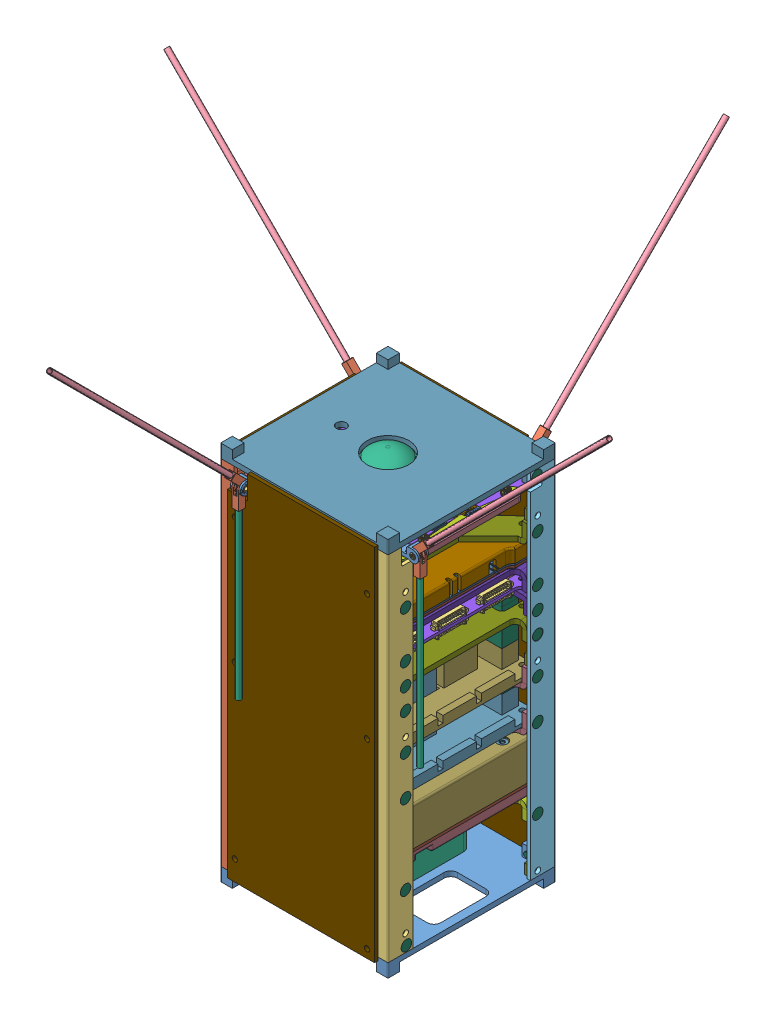
SolidWorks assembly Cubesat, configuration Default. Lengths in mm. (continued)
Mates (geometry in assembly coordinates):
- Coincident3: coincident: point of Cover Plate Bottom-1; point of assembly
- Coincident4: coincident: plane of Cover Plate Bottom-1 through (0 0 0) normal (0 -1 0); plane of assembly through (0 0 0) normal (0 1 0)
- Coincident5: coincident: plane of Cover Plate Bottom-1 through (0 0 0) normal (0 0 1); plane of assembly through (0 0 0) normal (0 0 1)
- Coincident7: coincident: plane of Cover Plate Bottom-1 through (0 0 0) normal (0 1 0); plane of Rail - Top Left-1 through (-50 0 -35) normal (0 -1 0)
- Coincident8: coincident: plane of Rail - Top Left-1 through (-50 211 -35) normal (0 0 1); plane of Cover Plate Bottom-1 through (-48 7 -35) normal (0 0 1)
- Coincident10: coincident: plane of Cover Plate Bottom-1 through (0 0 0) normal (0 1 0); plane of Rail - Top Right-1 through (35 0 -35) normal (0 -1 0)
- Coincident12: coincident: plane of Cover Plate Bottom-1 through (43 7 -48) normal (0 0 -1); plane of Rail - Top Right-1 through (35 211 -48) normal (0 0 1)
- Coincident13: coincident: plane of Cover Plate Bottom-1 through (0 0 0) normal (0 1 0); plane of Rail - Bottom Left-1 through (-50 0 50) normal (0 -1 0)
- Coincident14: coincident: plane of Cover Plate Bottom-1 through (-35 7 48) normal (0 0 1); plane of Rail - Bottom Left-1 through (-50 211 48) normal (0 0 -1)
- Coincident16: coincident: plane of Cover Plate Bottom-1 through (0 0 0) normal (0 1 0); plane of Rail - Bottom Right-1 through (50 0 50) normal (0 -1 0)
- Coincident18: coincident: plane of Rail - Bottom Right-1 through (50 211 35) normal (0 0 -1); plane of Cover Plate Bottom-1 through (48 7 35) normal (0 0 -1)
- Concentric1: concentric: circle of Camera-1; cylinder of Camera Plate - 4 tabs - bottom-1 through (-22.0002 39.32 -22.0002) axis (0 1 0) radius 1.7
- Concentric2: concentric: cylinder of Camera-1 through (22.0002 28.82 22.0002) axis (0 1 0) radius 1.5; cylinder of Camera Plate - 4 tabs - bottom-1 through (22.0002 39.32 22.0002) axis (0 1 0) radius 1.7
- Coincident19: coincident: plane of Camera-1 through (0 36.32 0) normal (0 1 0); plane of Camera Plate - 4 tabs - bottom-1 through (0 36.32 0) normal (0 -1 0)
- Concentric4: concentric: cylinder of Cover Plate Bottom-1 through (0 -3 0) axis (0 1 0) radius 12.5; cylinder of Camera-1 through (0 9.82 0) axis (0 1 0) radius 11.5307
- Distance2: distance = 2 mm: plane of Camera-1 through (0 -6 0) normal (0 -1 0); plane of Cover Plate Bottom-1 through (0 -8 0) normal (0 -1 0)
- Coincident30: coincident: plane of Camera Plate - 4 tabs - bottom-1 through (0 39.32 0) normal (0 1 0); plane of EPS1+-1/EPS1+.STEP-1/bottom-cover_Rev1.2.STEP-1 through (0 39.32 0) normal (0 -1 0)
- Concentric6: concentric: circle of Camera Plate - 4 tabs - bottom-1; circle of EPS1+-1/EPS1+.STEP-1/top-cover.STEP-1
- Concentric7: concentric: circle of Camera Plate - 4 tabs - bottom-1; circle of EPS1+-1/EPS1+.STEP-1/top-cover.STEP-1
- Coincident33: coincident: plane of Rail - Top Left-1 through (-48 211 -35) normal (1 0 0); plane of Camera Plate - 4 tabs - bottom-1 through (-48 39.32 0) normal (-1 0 0)
- Coincident37: coincident: plane of Camera-2 through (0 174.68 0) normal (0 -1 0); plane of Camera Plate - 4 tabs - top-1 through (0 174.68 0) normal (0 1 0)
- Coincident40: coincident: plane of Rail - Top Left-1 through (-48 211 -35) normal (1 0 0); plane of Camera Plate - 4 tabs - top-1 through (-48 174.68 0) normal (-1 0 0)
- Concentric10: concentric: cylinder of Camera-2 through (-22.0002 182.18 -22.0002) axis (0 -1 0) radius 1.5; cylinder of Camera Plate - 4 tabs - top-1 through (-22.0002 171.68 -22.0002) axis (0 1 0) radius 1.55
- Concentric13: concentric: circle of Camera Plate - 4 tabs - top-1; circle of OBC_EnduroSat-1/OBC_EnduroSat.STEP-1/Board021117.STEP-1
- Concentric14: concentric: cylinder of Camera Plate - 4 tabs - top-1 through (37.5 171.68 -42.85) axis (0 1 0) radius 1.55; circle of OBC_EnduroSat-1/OBC_EnduroSat.STEP-1/Board021117.STEP-1
- Concentric15: concentric: cylinder of Camera Plate - 4 tabs - top-1 through (-36.2 171.68 -42.85) axis (0 1 0) radius 1.55; cylinder of UHF_comm_type_II-1/UHF_comm_type_II.STEP-1/UHF_BOX.STEP-1 through (-36.2 168.68 -42.85) axis (0 -1 0) radius 1.6
- Concentric16: concentric: cylinder of Camera Plate - 4 tabs - top-1 through (37.5 171.68 -42.85) axis (0 1 0) radius 1.55; cylinder of UHF_comm_type_II-1/UHF_comm_type_II.STEP-1/UHF_BOX.STEP-1 through (37.5 168.68 -42.85) axis (0 -1 0) radius 1.6
- Distance4: distance = 24 mm: plane of OBC_EnduroSat-1/OBC_EnduroSat.STEP-1/Board021117.STEP-1 through (42.1 144.68 47.95) normal (0 -1 0); plane of UHF_comm_type_II-1/UHF_comm_type_II.STEP-1/UHF_BOX.STEP-1 through (40.1038 168.68 -45.05) normal (0 1 0)
- Distance5: distance = 6 mm: plane of UHF_comm_type_II-1/UHF_comm_type_II.STEP-1/UHF_BOX.STEP-1 through (40.1038 168.68 -45.05) normal (0 1 0); plane of Camera-2 through (0 174.68 0) normal (0 -1 0)
- Concentric17: concentric: cylinder of Custom Board 2-1 through (-36.2 77.989 -42.85) axis (0 -1 0) radius 1.6; cylinder of Custom Board 1 Plate-2 through (-36.2 72.989 -42.85) axis (0 1 0) radius 1.55
- Concentric18: concentric: cylinder of Custom Board 2-1 through (40 77.989 42.85) axis (0 -1 0) radius 1.6; circle of Custom Board 1 Plate-2
- Coincident49: coincident: plane of Custom Board 2-1 through (0 75.989 0) normal (0 -1 0); plane of Custom Board 1 Plate-2 through (0 75.989 0) normal (0 1 0)
- Concentric19: concentric: circle of Custom Board 1-1; cylinder of Custom Board 1 Plate-1 through (-36.2 96.589 -42.85) axis (0 1 0) radius 1.55
- Concentric20: concentric: cylinder of Custom Board 1-1 through (40 101.589 42.85) axis (0 -1 0) radius 1.6; cylinder of Custom Board 1 Plate-1 through (40 96.589 42.85) axis (0 1 0) radius 1.55
- Coincident51: coincident: plane of Custom Board 1-1 through (0 99.589 0) normal (0 -1 0); plane of Custom Board 1 Plate-1 through (0 99.589 0) normal (0 1 0)
- Coincident54: coincident: plane of EPS1+-1/EPS1+.STEP-1/ESQ_126_69_G_D.STEP-1/_ESQ_126_69_G_D_socket_2.STEP-1 through (-32.6249 65.189 -36.5581) normal (0 1 0); plane of PC104 Connector-1 through (-32.6269 65.189 -34.0211) normal (0 -1 0)
- Coincident55: coincident: plane of EPS1+-1/EPS1+.STEP-1/ESQ_126_69_G_D.STEP-2/_ESQ_126_69_G_D_socket_2.STEP-1 through (33.9231 65.189 -44.0511) normal (0 0 -1); plane of PC104 Connector-1 through (-32.6269 75.989 -44.0511) normal (0 0 -1)
- Coincident56: coincident: plane of EPS1+-1/EPS1+.STEP-1/ESQ_126_69_G_D.STEP-2/_ESQ_126_69_G_D_socket_2.STEP-1 through (33.9231 65.189 -39.0981) normal (1 0 0); plane of PC104 Connector-1 through (33.9231 75.989 -34.0211) normal (1 0 0)
- Concentric21: concentric: circle of EPS1+-1/EPS1+.STEP-1/top-cover.STEP-1; cylinder of Custom Board 2-1 through (37.5 77.989 -42.85) axis (0 -1 0) radius 1.6
- Coincident58: coincident: plane of Rail - Bottom Left-1 through (-48 211 50) normal (1 0 0); plane of Custom Board 1 Plate-2 through (-48 75.989 0) normal (-1 0 0)
- Coincident63: coincident: plane of Custom Board 2-1 through (0 75.989 0) normal (0 -1 0); plane of PC104 Connector-1 through (-32.6269 75.989 -34.0211) normal (0 1 0)
- Concentric22: concentric: circle of Custom Board 1-1; circle of Custom Board 2-1
- Coincident61: coincident: plane of Rail - Bottom Left-1 through (-48 211 50) normal (1 0 0); plane of Custom Board 1 Plate-1 through (-48 99.589 0) normal (-1 0 0)
- Coincident64: coincident: plane of Custom Board 2-1 through (0 88.789 0) normal (0 1 0); plane of PC104 Connector-2 through (-32.627 88.789 -34.051) normal (0 -1 0)
- Coincident65: coincident: plane of Custom Board 2-1 through (33.923 88.789 -44.081) normal (1 0 0); plane of PC104 Connector-2 through (33.923 99.589 -34.051) normal (1 0 0)
- Coincident66: coincident: plane of Custom Board 2-1 through (-32.625 88.789 -44.081) normal (0 0 -1); plane of PC104 Connector-2 through (-32.627 99.589 -44.081) normal (0 0 -1)
- Coincident67: coincident: plane of Custom Board 1-1 through (0 99.589 0) normal (0 -1 0); plane of PC104 Connector-2 through (-32.627 99.589 -34.051) normal (0 1 0)
- Coincident70: coincident: plane of Custom Board 1-1 through (0 112.389 0) normal (0 1 0); plane of PC104 Connector-4 through (-32.627 112.389 -34.112) normal (0 -1 0)
- Coincident71: coincident: plane of Custom Board 1-1 through (33.923 112.389 -44.091) normal (1 0 0); plane of PC104 Connector-4 through (33.923 123.189 -34.112) normal (1 0 0)
- Coincident73: coincident: plane of Custom Board 1-1 through (-32.625 112.389 -34.112) normal (0 0 1); plane of PC104 Connector-4 through (-32.627 123.189 -34.112) normal (0 0 1)
- Coincident74: coincident: plane of PC104 Connector-4 through (-32.627 123.189 -34.112) normal (0 1 0); plane of PC104 Connector-5 through (-32.627 123.189 -34.112) normal (0 -1 0)
- Coincident75: coincident: plane of PC104 Connector-4 through (33.923 123.189 -34.112) normal (1 0 0); plane of PC104 Connector-5 through (33.923 133.989 -34.112) normal (1 0 0)
- Coincident76: coincident: plane of Custom Board 1-1 through (-32.625 112.389 -34.112) normal (0 0 1); plane of PC104 Connector-5 through (-32.627 133.989 -34.112) normal (0 0 1)
- Coincident77: coincident: plane of PC104 Connector-3 through (-32.627 133.989 -34.112) normal (0 -1 0); plane of PC104 Connector-5 through (-32.627 133.989 -34.112) normal (0 1 0)
- Coincident78: coincident: plane of PC104 Connector-3 through (33.923 144.789 -34.112) normal (1 0 0); plane of PC104 Connector-5 through (33.923 133.989 -34.112) normal (1 0 0)
- Coincident79: coincident: plane of PC104 Connector-3 through (-32.627 144.789 -44.142) normal (0 0 -1); plane of PC104 Connector-5 through (-32.627 133.989 -44.142) normal (0 0 -1)
- Coincident82: coincident: plane of Rail - Top Left-1 through (-48 211 -35) normal (1 0 0); plane of Engraving plate-1 through (-48 131.989 0) normal (-1 0 0)
- Concentric25: concentric: cylinder of Custom Board 1-1 through (40 101.589 42.85) axis (0 -1 0) radius 1.6; circle of Engraving plate-1
- Distance7: distance = 1 mm: plane of Custom Board 2-1 through (0 127.989 0) normal (0 1 0); plane of Engraving plate-1 through (0 128.989 0) normal (0 -1 0)
- Coincident84: coincident: plane of Rail - Bottom Left-1 through (-48 211 50) normal (1 0 0); plane of OBC Board Plate-1 through (-48 144.68 0) normal (-1 0 0)
- Coincident85: coincident: plane of OBC_EnduroSat-1/OBC_EnduroSat.STEP-1/Board021117.STEP-1 through (42.1 144.68 47.95) normal (0 -1 0); plane of OBC Board Plate-1 through (0 144.68 0) normal (0 1 0)
- Concentric27: concentric: circle of Engraving plate-1; circle of Engraving-1
- Concentric28: concentric: circle of Engraving plate-1; circle of Engraving-1
- Coincident86: coincident: plane of Engraving plate-1 through (0 131.989 0) normal (0 1 0); plane of Engraving-1 through (0 131.989 0) normal (0 -1 0)
- Concentric30: concentric: circle of gs-3dcad-nanocom-ant430-2u3u-deployed-4-1/panel-top_ant430-2U-4-1; circle of Antenna Plate-1
- Concentric31: concentric: cylinder of gs-3dcad-nanocom-ant430-2u3u-deployed-4-1/2.5x4.5x3.0mm-spacer_ant430-2U-4-4 through (-45.8 206 24.7) axis (0 -1 0) radius 1.25; cylinder of Antenna Plate-1 through (-45.8 192 24.7) axis (0 1 0) radius 1.35
- Coincident87: coincident: plane of gs-3dcad-nanocom-ant430-2u3u-deployed-4-1/panel-top_ant430-2U-4-1 through (47.4 202 -32.35) normal (0 -1 0); plane of Antenna Plate-1 through (0 202 0) normal (0 1 0)
- Coincident88: coincident: plane of Rail - Bottom Left-1 through (-50 211 48) normal (0 0 -1); plane of Antenna Plate-1 through (0 202 48) normal (0 0 1)
- Coincident110: coincident: plane of Rail - Bottom Right-1 through (50 211 50) normal (0 1 0); plane of Cover Plate Top-2 through (0 211 0) normal (0 -1 0)
- Coincident111: coincident: plane of Rail - Bottom Right-1 through (50 211 48) normal (0 0 -1); plane of Cover Plate Top-2 through (35 204 48) normal (0 0 1)
- Coincident112: coincident: plane of Rail - Top Right-1 through (48 211 -35) normal (-1 0 0); plane of Cover Plate Top-2 through (48 204 -35) normal (1 0 0)
- Coincident113: coincident: plane of Rail - Bottom Right-1 through (35 211 50) normal (-1 0 0); plane of Antenna Plate-1 through (35 192 48) normal (-1 0 0)
- Concentric32: concentric: cone of Rail - Bottom Left-1 through (-50 178.5483 39.5) axis (1 0 0); cone of M3 Flathead-3 through (-50 178.5483 39.5) axis (1 0 0)
- Coincident116: coincident: circle of Rail - Bottom Left-1; cone of M3 Flathead-1 through (-50 150.8117 39.5) axis (1 0 0)
- Coincident117: coincident: circle of Rail - Bottom Left-1; circle of M3 Flathead-8
- Coincident118: coincident: circle of Rail - Bottom Left-1; circle of M3 Flathead-5
- Coincident119: coincident: circle of Rail - Bottom Left-1; circle of M3 Flathead-7
- Coincident120: coincident: circle of Rail - Bottom Left-1; circle of M3 Flathead-2
- Coincident121: coincident: circle of Rail - Top Left-1; cone of M3 Flathead-6 through (-50 178.5483 -39.5) axis (1 0 0)
- Coincident122: coincident: circle of Rail - Top Left-1; cone of M3 Flathead-4 through (-49.8242 150.8117 -39.5) axis (1 0 0)
- Concentric33: concentric: cone of Rail - Top Left-1 through (-50 137.8117 -39.5) axis (1 0 0); cone of M3 Flathead-12 through (-50 137.8117 -39.5) axis (1 0 0)
- Coincident124: coincident: circle of Rail - Top Left-1; circle of M3 Flathead-11
- Coincident125: coincident: circle of Rail - Top Left-1; circle of M3 Flathead-9
- Coincident126: coincident: circle of Rail - Top Left-1; circle of M3 Flathead-10
- Coincident127: coincident: circle of Rail - Top Left-1; circle of M3 Flathead-13
- Coincident128: coincident: circle of Rail - Bottom Right-1; circle of M3 Flathead-14
- Coincident129: coincident: circle of Rail - Top Right-1; circle of M3 Flathead-15
- Coincident130: coincident: circle of Rail - Bottom Right-1; circle of M3 Flathead-16
- Coincident131: coincident: circle of Rail - Top Right-1; circle of M3 Flathead-17
- Coincident132: coincident: circle of Rail - Bottom Right-1; circle of M3 Flathead-18
- Coincident133: coincident: circle of Rail - Top Right-1; circle of M3 Flathead-19
- Coincident134: coincident: circle of Rail - Bottom Right-1; circle of M3 Flathead-20
- Coincident135: coincident: circle of Rail - Top Right-1; cone of M3 Flathead-21 through (49.8242 125.1207 -39.5) axis (-1 0 0)
- Coincident136: coincident: cone of Rail - Bottom Right-1 through (50 103.5207 39.5) axis (-1 0 0); circle of M3 Flathead-22
- Concentric34: concentric: cone of Rail - Top Right-1 through (50 103.4607 -39.5) axis (-1 0 0); cone of M3 Flathead-23 through (50 103.4607 -39.5) axis (-1 0 0)
- Coincident137: coincident: circle of Rail - Bottom Right-1; circle of M3 Flathead-24
- Coincident138: coincident: circle of Rail - Top Right-1; circle of M3 Flathead-26
- Concentric36: concentric: cone of Rail - Bottom Right-1 through (50 32.5107 39.5) axis (-1 0 0); cone of M3 Flathead-25 through (50 32.5107 39.5) axis (-1 0 0)
- Concentric38: concentric: cone of Rail - Top Left-1 through (-39 207.5 -50) axis (0 0 1); cone of M3 Flathead-28 through (-39 207.5 -50) axis (0 0 1)
- Concentric39: concentric: cone of Rail - Bottom Left-1 through (-50 207.5 39) axis (1 0 0); cone of M3 Flathead-29 through (-50 207.5 39) axis (1 0 0)
- Concentric40: concentric: cone of Rail - Top Right-1 through (50 207.5 -39) axis (-1 0 0); cone of M3 Flathead-30 through (50 207.5 -39) axis (-1 0 0)
- Concentric41: concentric: cone of Rail - Bottom Right-1 through (39 207.5 50) axis (0 0 -1); cone of M3 Flathead-31 through (39 207.5 50) axis (0 0 -1)
- Coincident139: coincident: plane of Rail - Bottom Right-1 through (50 211 35) normal (0 0 -1); plane of Cover Plate Bottom-1 through (48 7 35) normal (0 0 -1)
- Coincident140: coincident: plane of Cover Plate Bottom-1 through (35 7 -48) normal (-1 0 0); plane of Rail - Top Right-1 through (35 211 -35) normal (-1 0 0)
- Concentric42: concentric: circle of Camera-2; circle of Camera Plate - 4 tabs - top-1
- Concentric43: concentric: cylinder of Camera Plate - 4 tabs - top-1 through (-40 171.68 42.85) axis (0 1 0) radius 1.55; cylinder of Engraving plate-1 through (-40 128.989 42.85) axis (0 1 0) radius 1.6
- Distance8: distance = 2 mm: plane of Camera-2 through (0 217 0) normal (0 1 0); plane of Cover Plate Top-2 through (0 219 0) normal (0 1 0)
- Concentric44: concentric: cylinder of Engraving plate-1 through (-40 128.989 42.85) axis (0 1 0) radius 1.6; cylinder of OBC Board Plate-1 through (-40 141.68 42.85) axis (0 1 0) radius 1.55
- Coincident141: coincident: cone of Rail - Top Right-1 through (50 32.4507 -39.5) axis (-1 0 0); circle of M3 Flathead-27
- Coincident142: coincident: plane of Cover Plate Bottom-1 through (48 7 35) normal (1 0 0); plane of Rail - Bottom Right-1 through (48 211 50) normal (-1 0 0)
- Distance9: distance = 1 mm: plane of Rail - Top Right-1 through (35 201 -35) normal (0 1 0); plane of gs-3dcad-nanocom-ant430-2u3u-deployed-4-1/panel-top_ant430-2U-4-1 through (47.4 202 -32.35) normal (0 -1 0)
- Coincident143: coincident: circle of Rail - Bottom Left-1; circle of M3 Flathead-32
- Coincident144: coincident: circle of Rail - Bottom Right-1; circle of M3 Flathead-33
- Coincident145: coincident: circle of Rail - Top Right-1; circle of M3 Flathead-34
- Coincident146: coincident: circle of Rail - Top Left-1; circle of M3 Flathead-35
- Coincident147: coincident: circle of Rail - Bottom Left-1; circle of M3 Flathead-36
- Coincident156: coincident: plane of Cover Plate Bottom-1 through (0 7 0) normal (0 1 0); plane of M3 Square Nut-29 through (48 7 42.5) normal (0 -1 0)
- Coincident157: coincident: plane of Cover Plate Bottom-1 through (0 0 0) normal (0 1 0); plane of M3 Square Nut-25 through (48 0 -36.5) normal (0 -1 0)
- Coincident158: coincident: plane of Custom Board 1 Plate-1 through (48 108.589 35) normal (0 1 0); plane of M3 Square Nut-30 through (48 108.589 36.5) normal (0 -1 0)
- Coincident160: coincident: plane of Camera Plate - 4 tabs - top-1 through (48 183.68 44) normal (0 1 0); plane of M3 Square Nut-32 through (48 183.68 42.5) normal (0 -1 0)
- Coincident161: coincident: plane of Camera Plate - 4 tabs - top-1 through (48 183.68 -35) normal (0 1 0); plane of M3 Square Nut-28 through (48 183.68 -36.5) normal (0 -1 0)
- Coincident163: coincident: plane of Custom Board 1 Plate-1 through (48 108.589 -44) normal (0 1 0); plane of M3 Square Nut-26 through (48 108.589 -36.5) normal (0 -1 0)
- Coincident164: coincident: plane of M3 Square Nut-21 through (-45 0 36.5) normal (0 -1 0); plane of Cover Plate Bottom-1 through (0 0 0) normal (0 1 0)
- Coincident165: coincident: plane of Cover Plate Bottom-1 through (0 7 0) normal (0 1 0); plane of M3 Square Nut-17 through (-48 7 -36.5) normal (0 -1 0)
- Coincident166: coincident: plane of Custom Board 1 Plate-1 through (-48 108.589 35) normal (0 1 0); plane of M3 Square Nut-22 through (-48 108.589 42.5) normal (0 -1 0)
- Coincident167: coincident: plane of Custom Board 1 Plate-1 through (-48 108.589 -35) normal (0 1 0); plane of M3 Square Nut-18 through (-48 108.589 -36.5) normal (0 -1 0)
- Coincident170: coincident: plane of Camera Plate - 4 tabs - top-1 through (-48 183.68 35) normal (0 1 0); plane of M3 Square Nut-24 through (-45 183.68 36.5) normal (0 -1 0)
- Coincident171: coincident: plane of Camera Plate - 4 tabs - top-1 through (-48 183.68 -44) normal (0 1 0); plane of M3 Square Nut-20 through (-48 183.68 -42.5) normal (0 -1 0)
- Coincident175: coincident: plane of Rail - Top Right-1 through (48 211 -35) normal (-1 0 0); plane of M3 Square Nut-28 through (48 183.68 -36.5) normal (1 0 0)
- Coincident176: coincident: plane of Camera Plate - 4 tabs - top-1 through (48 174.68 0) normal (1 0 0); plane of M3 Square Nut-32 through (48 183.68 42.5) normal (1 0 0)
- Coincident179: coincident: plane of Custom Board 1 Plate-2 through (48 75.989 0) normal (1 0 0); plane of M3 Square Nut-30 through (48 114.589 36.5) normal (1 0 0)
- Coincident180: coincident: plane of Rail - Top Right-1 through (48 211 -35) normal (-1 0 0); plane of M3 Square Nut-26 through (48 114.589 -36.5) normal (1 0 0)
- Coincident181: coincident: plane of Cover Plate Bottom-1 through (48 7 35) normal (1 0 0); plane of M3 Square Nut-29 through (48 13 42.5) normal (1 0 0)
- Coincident182: coincident: plane of Rail - Top Right-1 through (48 211 -35) normal (-1 0 0); plane of M3 Square Nut-25 through (48 0 -36.5) normal (1 0 0)
- Coincident183: coincident: plane of UHF_comm_type_II-1/UHF_comm_type_II.STEP-1/UHF_BOX-bottom-part(nif).STEP-1 through (44.4 157.68 33.95) normal (0 -1 0); plane of Custom Plate - tabs down-1 through (0 157.68 0) normal (0 1 0)
- Concentric47: concentric: cylinder of UHF_comm_type_II-1/UHF_comm_type_II.STEP-1/UHF_BOX-bottom-part(nif).STEP-1 through (-40 159.68 42.85) axis (0 -1 0) radius 1.6; cylinder of Custom Plate - tabs down-1 through (-40 154.68 42.85) axis (0 1 0) radius 1.55
- Concentric48: concentric: cylinder of UHF_comm_type_II-1/UHF_comm_type_II.STEP-1/UHF_BOX-bottom-part(nif).STEP-1 through (-36.2 157.68 -42.85) axis (0 1 0) radius 1.6; circle of Custom Plate - tabs down-1
- Coincident184: coincident: plane of Rail - Top Left-1 through (-48 211 -35) normal (1 0 0); plane of M3 Square Nut-17 through (-48 7 -36.5) normal (-1 0 0)
- Coincident185: coincident: plane of M3 Square Nut-17 through (-48 7 -36.5) normal (-1 0 0); plane of M3 Square Nut-21 through (-48 6 36.5) normal (-1 0 0)
- Coincident186: coincident: plane of Custom Board 1 Plate-1 through (-48 99.589 0) normal (-1 0 0); plane of M3 Square Nut-22 through (-48 114.589 42.5) normal (-1 0 0)
- Coincident187: coincident: plane of Custom Board 1 Plate-1 through (-48 99.589 0) normal (-1 0 0); plane of M3 Square Nut-18 through (-48 114.589 -36.5) normal (-1 0 0)
- Concentric53: concentric: cylinder of Rail - Bottom Right-1 through (40 10 39.5) axis (1 0 0) radius 1.7; cylinder of M3 Square Nut-29 through (48 10 39.5) axis (-1 0 0) radius 1.6
- Concentric55: concentric: cylinder of Rail - Top Right-1 through (40 3 -39.5) axis (1 0 0) radius 1.7; cylinder of M3 Square Nut-25 through (48 3 -39.5) axis (-1 0 0) radius 1.6
- Concentric56: concentric: cylinder of Rail - Bottom Left-1 through (-40 3 39.5) axis (-1 0 0) radius 1.7; cylinder of M3 Square Nut-21 through (-45 3 39.5) axis (-1 0 0) radius 1.6
- Concentric57: concentric: cylinder of Rail - Top Left-1 through (-40 10 -39.5) axis (-1 0 0) radius 1.7; cylinder of M3 Square Nut-17 through (-48 10 -39.5) axis (1 0 0) radius 1.6
- Coincident189: coincident: plane of Rail - Bottom Left-1 through (-48 211 50) normal (1 0 0); plane of M3 Square Nut-24 through (-48 183.68 36.5) normal (-1 0 0)
- Coincident195: coincident: plane of Rail - Bottom Right-1 through (50 211 50) normal (0 0 1); plane of Solar panel plate-2 through (-44 -2 50) normal (0 0 -1)
- Distance10: distance = 1 mm: plane of Cover Plate Top-2 through (0 214 0) normal (0 1 0); plane of Solar panel plate-2 through (-44 213 52) normal (0 1 0)
- Distance11: distance = 1 mm: plane of Cover Plate Bottom-1 through (-43 -8 50) normal (1 0 0); plane of Solar panel plate-2 through (-44 -2 52) normal (-1 0 0)
- Coincident198: coincident: plane of Rail - Bottom Left-1 through (-50 211 50) normal (-1 0 0); plane of Solar panel plate-4 through (-50 -2 -44) normal (1 0 0)
- Concentric67: concentric: circle of Rail - Top Left-1; circle of Solar panel plate-4
- Concentric68: concentric: circle of Rail - Bottom Left-1; circle of Solar panel plate-4
- Coincident201: coincident: plane of Rail - Top Right-1 through (35 211 -50) normal (0 0 -1); plane of Solar panel plate-3 through (44 -2 -50) normal (0 0 1)
- Concentric70: concentric: circle of Rail - Top Right-1; circle of Solar panel plate-3
- Concentric71: concentric: circle of Rail - Top Left-1; circle of Solar panel plate-3
- Coincident203: coincident: plane of Rail - Bottom Right-1 through (50 211 50) normal (1 0 0); plane of Solar panel plate-5 through (50 -2 44) normal (-1 0 0)
- Concentric72: concentric: cylinder of Rail - Top Right-1 through (40 186.68 -39.5) axis (1 0 0) radius 1.7; circle of Solar panel plate-5
- Concentric73: concentric: cylinder of Rail - Bottom Right-1 through (40 186.68 39.5) axis (1 0 0) radius 1.7; cylinder of Solar panel plate-5 through (52 186.68 39.5) axis (-1 0 0) radius 1.6
- Coincident204: coincident: plane of gs-3dcad-nanocom-ant430-2u3u-deployed-4-1/antenna-assembly-top-2U-4.0_ant430-2U-4(Deployed)-2-1/antenna-bracket-top-2_ant430-2U-4-1 through (51.2503 209.2 35) normal (0 1 0); plane of gs-3dcad-nanocom-ant430-1u-stowed-4-1/antenna-assembly-top-2U-4.0_ant430-1U-4(Default - Stowed)-1-1/antenna-bracket-top-2_ant430-1U-4-1 through (-51.2503 209.2 -35) normal (0 1 0)
- Concentric74: concentric: cylinder of gs-3dcad-nanocom-ant430-2u3u-deployed-4-1/2.5x4.5x3.0mm-spacer_ant430-2U-4-3 through (45.8 206 -24.7) axis (0 -1 0) radius 1.25; cylinder of gs-3dcad-nanocom-ant430-1u-stowed-4-1/2.5x4.5x3.0mm-spacer_ant430-1U-4-4 through (45.8 206 -24.7) axis (0 -1 0) radius 1.25
- Concentric75: concentric: cylinder of gs-3dcad-nanocom-ant430-2u3u-deployed-4-1/2.5x4.5x3.0mm-spacer_ant430-2U-4-4 through (-45.8 206 24.7) axis (0 -1 0) radius 1.25; cylinder of gs-3dcad-nanocom-ant430-1u-stowed-4-1/2.5x4.5x3.0mm-spacer_ant430-1U-4-3 through (-45.8 206 24.7) axis (0 -1 0) radius 1.25
